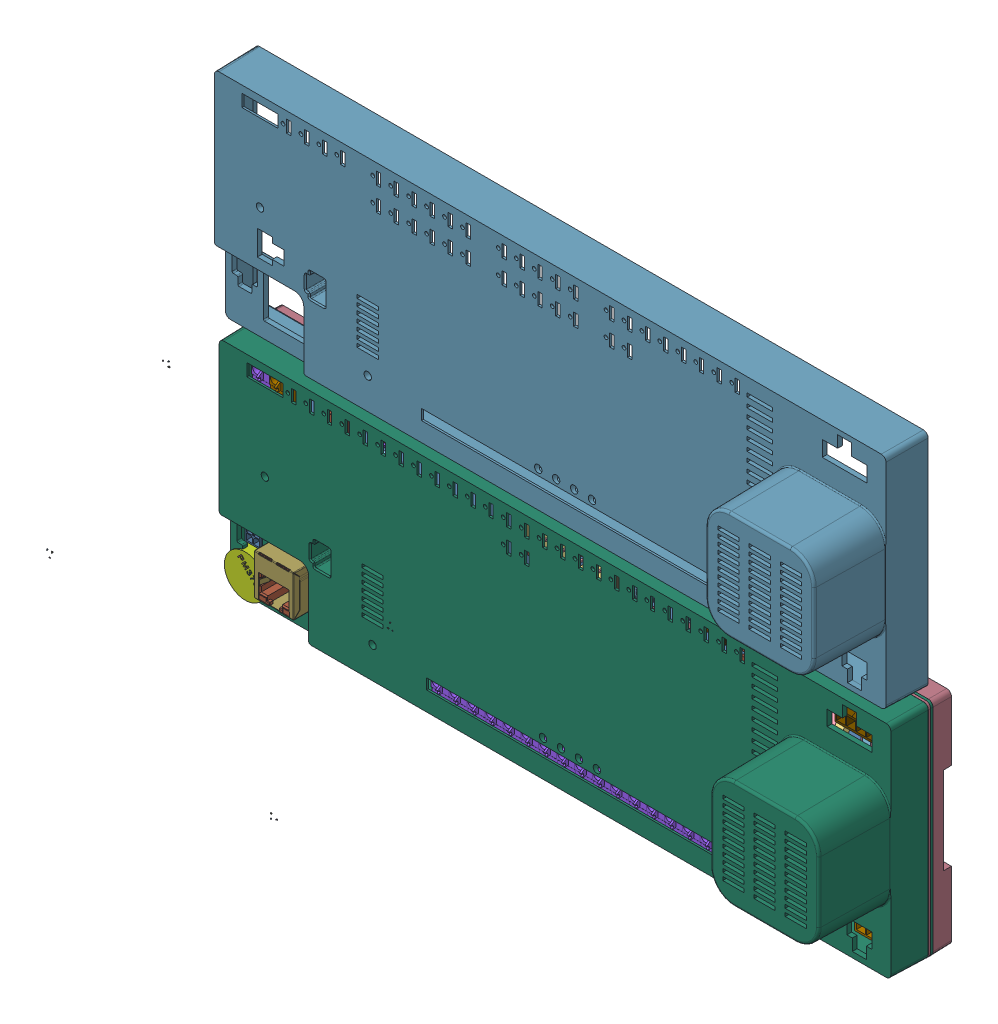
SolidWorks assembly _SC944D, configuration Default. Lengths in mm. (continued)
Components (placement in the parent): (continued)
- R2-1: R2 [Default] at origin size (0.8 1.6 0.55)
  - RESC1608X84N-1: RESC1608X84N [Default] at (41.4337 68.2626 0) x (0 1 0) z (1 0 0) size (1.6 0.55 0.8)
- R3-1: R3 [Default] at origin size (1.6 0.8 0.55)
  - RESC1608X84N-1: RESC1608X84N [Default] at (55.5308 79.4703 0) x (1 0 0) z (0 -1 0) size (1.6 0.55 0.8)
- R4-1: R4 [Default] at origin size (1.6 0.8 0.55)
  - RESC1608X84N-1: RESC1608X84N [Default] at (43.8151 70.9613 0) x (1 0 0) z (0 -1 0) size (1.6 0.55 0.8)
- R5-1: R5 [Default] at origin size (1.6 0.8 0.55)
  - RESC1608X84N-1: RESC1608X84N [Default] at (83.0262 24.4474 0) x (-1 0 0) z (0 1 0) size (1.6 0.55 0.8)
- R6-1: R6 [Default] at origin size (1.6 0.8 0.55)
  - RESC1608X84N-1: RESC1608X84N [Default] at (39.6876 53.8163 0) x (1 0 0) z (0 -1 0) size (1.6 0.55 0.8)
- R7-1: R7 [Default] at origin size (1.6 0.8 0.55)
  - RESC1608X84N-1: RESC1608X84N [Default] at (97.4091 78.7401 0) x (1 0 0) z (0 -1 0) size (1.6 0.55 0.8)
- R8-1: R8 [Default] at origin size (1.6 0.8 0.55)
  - RESC1608X84N-1: RESC1608X84N [Default] at (97.4089 76.9619 0) x (-1 0 0) z (0 1 0) size (1.6 0.55 0.8)
- R9-1: R9 [Default] at origin size (3.2 1.6 0.84)
  - RESC3216X84N-1: RESC3216X84N [Default] at (57.7849 61.1187 0) x (-1 0 0) z (0 1 0) size (3.2 0.84 1.6)
- R10-1: R10 [Default] at origin size (1.6 0.8 0.55)
  - RESC1608X84N-1: RESC1608X84N [Default] at (29.2099 4.2862 0) x (-1 0 0) z (0 1 0) size (1.6 0.55 0.8)
- R11-1: R11 [Default] at origin size (1.6 0.8 0.55)
  - RESC1608X84N-1: RESC1608X84N [Default] at (146.0499 57.5309 0) x (-1 0 0) z (0 1 0) size (1.6 0.55 0.8)
- R12-1: R12 [Default] at origin size (1.6 0.8 0.55)
  - RESC1608X84N-1: RESC1608X84N [Default] at (115.0619 55.7529 0) x (-1 0 0) z (0 1 0) size (1.6 0.55 0.8)
- R14-1: R14 [Default] at origin size (1.6 0.8 0.55)
  - RESC1608X84N-1: RESC1608X84N [Default] at (120.7769 63.2459 0) x (-1 0 0) z (0 1 0) size (1.6 0.55 0.8)
- R15-1: R15 [Default] at origin size (0.8 1.6 0.55)
  - RESC1608X84N-1: RESC1608X84N [Default] at (118.3641 63.8809 0) x (0 -1 0) z (-1 0 0) size (1.6 0.55 0.8)
- R16-1: R16 [Default] at origin size (1.6 0.8 0.55)
  - RESC1608X84N-1: RESC1608X84N [Default] at (29.2099 2.5399 0) x (-1 0 0) z (0 1 0) size (1.6 0.55 0.8)
- R17-1: R17 [Default] at origin size (1.6 0.8 0.55)
  - RESC1608X84N-1: RESC1608X84N [Default] at (143.3831 50.6731 0) x (1 0 0) z (0 -1 0) size (1.6 0.55 0.8)
- R18-1: R18 [Default] at origin size (0.8 1.6 0.55)
  - RESC1608X84N-1: RESC1608X84N [Default] at (121.6661 53.7209 0) x (0 -1 0) z (-1 0 0) size (1.6 0.55 0.8)
- R19-1: R19 [Default] at origin size (3.2 1.6 0.84)
  - RESC3216X84N-1: RESC3216X84N [Default] at (110.1724 8.8899 0) x (-1 0 0) z (0 1 0) size (3.2 0.84 1.6)
- R20-1: R20 [Default] at origin size (3.2 1.6 0.84)
  - RESC3216X84N-1: RESC3216X84N [Default] at (110.2359 24.7649 0) x (-1 0 0) z (0 1 0) size (3.2 0.84 1.6)
- R21-1: R21 [Default] at origin size (1.6 0.8 0.55)
  - RESC1608X84N-1: RESC1608X84N [Default] at (119.1261 50.4191 0) x (1 0 0) z (0 -1 0) size (1.6 0.55 0.8)
- R22-1: R22 [Default] at origin size (1.6 0.8 0.55)
  - RESC1608X84N-1: RESC1608X84N [Default] at (39.6874 61.2775 0) x (-1 0 0) z (0 1 0) size (1.6 0.55 0.8)
- R23-1: R23 [Default] at origin size (1.6 0.8 0.55)
  - RESC1608X84N-1: RESC1608X84N [Default] at (200.5649 35.4012 0) x (-1 0 0) z (0 1 0) size (1.6 0.55 0.8)
- R24-1: R24 [Default] at origin size (6.4 3.2 0.7)
  - RESC6432X76N-1: RESC6432X76N [Default] at (160.782 62.4839 0) x (-1 0 0) z (0 1 0) size (6.4 0.7 3.2)
- R25-1: R25 [Default] at origin size (0.8 1.6 0.55)
  - RESC1608X84N-1: RESC1608X84N [Default] at (162.0521 66.6749 0) x (0 -1 0) z (-1 0 0) size (1.6 0.55 0.8)
- R26-1: R26 [Default] at origin size (1.6 0.8 0.55)
  - RESC1608X84N-1: RESC1608X84N [Default] at (162.6869 73.5329 0) x (-1 0 0) z (0 1 0) size (1.6 0.55 0.8)
- R27-1: R27 [Default] at origin size (0.8 1.6 0.55)
  - RESC1608X84N-1: RESC1608X84N [Default] at (80.3276 25.0824 0) x (0 -1 0) z (-1 0 0) size (1.6 0.55 0.8)
- R28-1: R28 [Default] at origin size (6.4 3.2 0.7)
  - RESC6432X76N-1: RESC6432X76N [Default] at (180.0861 65.9131 0) x (1 0 0) z (0 -1 0) size (6.4 0.7 3.2)
- R29-1: R29 [Default] at origin size (1.6 0.8 0.55)
  - RESC1608X84N-1: RESC1608X84N [Default] at (186.0549 70.866 0) x (-1 0 0) z (0 1 0) size (1.6 0.55 0.8)
- R30-1: R30 [Default] at origin size (1.6 0.8 0.55)
  - RESC1608X84N-1: RESC1608X84N [Default] at (189.1029 70.866 0) x (-1 0 0) z (0 1 0) size (1.6 0.55 0.8)
- R31-1: R31 [Default] at origin size (0.8 1.6 0.55)
  - RESC1608X84N-1: RESC1608X84N [Default] at (35.0838 21.4312 0) x (0 -1 0) z (-1 0 0) size (1.6 0.55 0.8)
- R32-1: R32 [Default] at origin size (1.6 0.8 0.55)
  - RESC1608X84N-1: RESC1608X84N [Default] at (82.8676 30.1626 0) x (1 0 0) z (0 -1 0) size (1.6 0.55 0.8)
- R33-1: R33 [Default] at origin size (0.8 1.6 0.55)
  - RESC1608X84N-1: RESC1608X84N [Default] at (57.9437 58.2613 0) x (0 1 0) z (1 0 0) size (1.6 0.55 0.8)
- R34-1: R34 [Default] at origin size (1.6 0.8 0.55)
  - RESC1608X84N-1: RESC1608X84N [Default] at (139.0649 50.7288 0) x (-1 0 0) z (0 1 0) size (1.6 0.55 0.8)
- R37-1: R37 [Default] at origin size (3.2 1.6 0.84)
  - RESC3216X84N-1: RESC3216X84N [Default] at (136.9059 57.9678 0) x (-1 0 0) z (0 1 0) size (3.2 0.84 1.6)
- R39-1: R39 [Default] at origin size (1.6 0.8 0.55)
  - RESC1608X84N-1: RESC1608X84N [Default] at (78.7401 11.7475 0) x (1 0 0) z (0 -1 0) size (1.6 0.55 0.8)
- R41-1: R41 [Default] at origin size (1.6 0.8 0.55)
  - RESC1608X84N-1: RESC1608X84N [Default] at (107.0609 27.8129 0) x (-1 0 0) z (0 1 0) size (1.6 0.55 0.8)
- R42-1: R42 [Default] at origin size (1.6 0.8 0.55)
  - RESC1608X84N-1: RESC1608X84N [Default] at (24.7649 33.9724 0) x (-1 0 0) z (0 1 0) size (1.6 0.55 0.8)
- R43-1: R43 [Default] at origin size (1.6 0.8 0.55)
  - RESC1608X84N-1: RESC1608X84N [Default] at (27.1462 51.435 0) x (-1 0 0) z (0 1 0) size (1.6 0.55 0.8)
- R44-1: R44 [Default] at origin size (0.8 1.6 0.55)
  - RESC1608X84N-1: RESC1608X84N [Default] at (28.5749 44.6088 0) x (0 1 0) z (1 0 0) size (1.6 0.55 0.8)
- R45-1: R45 [Default] at origin size (1.6 0.8 0.55)
  - RESC1608X84N-1: RESC1608X84N [Default] at (36.6712 53.8162 0) x (-1 0 0) z (0 1 0) size (1.6 0.55 0.8)
- R46-1: R46 [Default] at origin size (1.6 0.8 0.55)
  - RESC1608X84N-1: RESC1608X84N [Default] at (31.5912 47.625 0) x (-1 0 0) z (0 1 0) size (1.6 0.55 0.8)
- R47-1: R47 [Default] at origin size (1.6 0.8 0.55)
  - RESC1608X84N-1: RESC1608X84N [Default] at (73.8188 20.955 0) x (1 0 0) z (0 -1 0) size (1.6 0.55 0.8)
- R48-1: R48 [Default] at origin size (1.6 0.8 0.55)
  - RESC1608X84N-1: RESC1608X84N [Default] at (67.1513 9.6838 0) x (1 0 0) z (0 -1 0) size (1.6 0.55 0.8)
- R49-1: R49 [Default] at origin size (1.6 0.8 0.55)
  - RESC1608X84N-1: RESC1608X84N [Default] at (9.0488 62.5475 0) x (1 0 0) z (0 -1 0) size (1.6 0.55 0.8)
- R50-1: R50 [Default] at origin size (0.8 1.6 0.55)
  - RESC1608X84N-1: RESC1608X84N [Default] at (33.3376 52.2287 0) x (0 -1 0) z (-1 0 0) size (1.6 0.55 0.8)
- R51-1: R51 [Default] at origin size (0.8 1.6 0.55)
  - RESC1608X84N-1: RESC1608X84N [Default] at (83.566 41.7831 0) x (0 1 0) z (1 0 0) size (1.6 0.55 0.8)
- R52-1: R52 [Default] at origin size (0.8 1.6 0.55)
  - RESC1608X84N-1: RESC1608X84N [Default] at (100.7109 38.9891 0) x (0 1 0) z (1 0 0) size (1.6 0.55 0.8)
- R53-1: R53 [Default] at origin size (1.6 0.8 0.55)
  - RESC1608X84N-1: RESC1608X84N [Default] at (21.9076 37.9413 0) x (1 0 0) z (0 -1 0) size (1.6 0.55 0.8)
- R54-1: R54 [Default] at origin size (1.6 0.8 0.55)
  - RESC1608X84N-1: RESC1608X84N [Default] at (170.5611 79.248 0) x (1 0 0) z (0 -1 0) size (1.6 0.55 0.8)
- R55-1: R55 [Default] at origin size (1.6 0.8 0.55)
  - RESC1608X84N-1: RESC1608X84N [Default] at (173.7361 77.47 0) x (1 0 0) z (0 -1 0) size (1.6 0.55 0.8)
- R56-1: R56 [Default] at origin size (1.6 0.8 0.55)
  - RESC1608X84N-1: RESC1608X84N [Default] at (233.3626 27.4638 0) x (1 0 0) z (0 -1 0) size (1.6 0.55 0.8)
- R57-1: R57 [Default] at origin size (0.8 1.6 0.55)
  - RESC1608X84N-1: RESC1608X84N [Default] at (83.566 48.5496 0) x (0 1 0) z (1 0 0) size (1.6 0.55 0.8)
- R58-1: R58 [Default] at origin size (1.6 0.8 0.55)
  - RESC1608X84N-1: RESC1608X84N [Default] at (103.5049 34.1629 0) x (-1 0 0) z (0 1 0) size (1.6 0.55 0.8)
- R59-1: R59 [Default] at origin size (0.8 1.6 0.55)
  - RESC1608X84N-1: RESC1608X84N [Default] at (189.8488 36.2305 0) x (0 -1 0) z (-1 0 0) size (1.6 0.55 0.8)
- R60-1: R60 [Default] at origin size (1.6 0.8 0.55)
  - RESC1608X84N-1: RESC1608X84N [Default] at (107.0609 34.1629 0) x (-1 0 0) z (0 1 0) size (1.6 0.55 0.8)
- R61-1: R61 [Default] at origin size (0.8 1.6 0.55)
  - RESC1608X84N-1: RESC1608X84N [Default] at (240.5062 77.3113 0) x (0 1 0) z (1 0 0) size (1.6 0.55 0.8)
- R62-1: R62 [Default] at origin size (0.8 1.6 0.55)
  - RESC1608X84N-1: RESC1608X84N [Default] at (11.4301 62.8649 0) x (0 -1 0) z (-1 0 0) size (1.6 0.55 0.8)
- R63-1: R63 [Default] at origin size (0.8 1.6 0.55)
  - RESC1608X84N-1: RESC1608X84N [Default] at (230.775 77.9781 0) x (0 1 0) z (1 0 0) size (1.6 0.55 0.8)
- R65-1: R65 [Default] at origin size (1.6 0.8 0.55)
  - RESC1608X84N-1: RESC1608X84N [Default] at (233.3624 25.8762 0) x (-1 0 0) z (0 1 0) size (1.6 0.55 0.8)
- R66-1: R66 [Default] at origin size (0.8 1.6 0.55)
  - RESC1608X84N-1: RESC1608X84N [Default] at (193.8337 52.7051 0) x (0 1 0) z (1 0 0) size (1.6 0.55 0.8)
- R67-1: R67 [Default] at origin size (1.6 0.8 0.55)
  - RESC1608X84N-1: RESC1608X84N [Default] at (243.0462 76.6762 0) x (-1 0 0) z (0 1 0) size (1.6 0.55 0.8)
- R68-1: R68 [Default] at origin size (1.6 0.8 0.55)
  - RESC1608X84N-1: RESC1608X84N [Default] at (244.4749 74.144 0) x (-1 0 0) z (0 1 0) size (1.6 0.55 0.8)
- R69-1: R69 [Default] at origin size (0.8 1.6 0.55)
  - RESC1608X84N-1: RESC1608X84N [Default] at (234.4738 72.0724 0) x (0 -1 0) z (-1 0 0) size (1.6 0.55 0.8)
- R70-1: R70 [Default] at origin size (1.6 0.8 0.55)
  - RESC1608X84N-1: RESC1608X84N [Default] at (230.8224 67.7862 0) x (-1 0 0) z (0 1 0) size (1.6 0.55 0.8)
- R71-1: R71 [Default] at origin size (0.8 1.6 0.55)
  - RESC1608X84N-1: RESC1608X84N [Default] at (36.8299 21.4313 0) x (0 1 0) z (1 0 0) size (1.6 0.55 0.8)
- R72-1: R72 [Default] at origin size (1.6 0.8 0.55)
  - RESC1608X84N-1: RESC1608X84N [Default] at (29.7179 18.161 0) x (-1 0 0) z (0 1 0) size (1.6 0.55 0.8)
- R73-1: R73 [Default] at origin size (1.6 0.8 0.55)
  - RESC1608X84N-1: RESC1608X84N [Default] at (37.0244 6.8263 0) x (1 0 0) z (0 -1 0) size (1.6 0.55 0.8)
- R74-1: R74 [Default] at origin size (0.8 1.6 0.55)
  - RESC1608X84N-1: RESC1608X84N [Default] at (202.7238 61.1187 0) x (0 -1 0) z (-1 0 0) size (1.6 0.55 0.8)
- R75-1: R75 [Default] at origin size (0.8 1.6 0.55)
  - RESC1608X84N-1: RESC1608X84N [Default] at (41.783 20.9549 0) x (0 -1 0) z (-1 0 0) size (1.6 0.55 0.8)
- R76-1: R76 [Default] at origin size (0.8 1.6 0.55)
  - RESC1608X84N-1: RESC1608X84N [Default] at (34.1313 44.1324 0) x (0 -1 0) z (-1 0 0) size (1.6 0.55 0.8)
- R77-1: R77 [Default] at origin size (1.6 0.8 0.55)
  - RESC1608X84N-1: RESC1608X84N [Default] at (29.7179 16.6369 0) x (-1 0 0) z (0 1 0) size (1.6 0.55 0.8)
- R78-1: R78 [Default] at origin size (1.6 0.8 0.55)
  - RESC1608X84N-1: RESC1608X84N [Default] at (29.7179 15.1129 0) x (-1 0 0) z (0 1 0) size (1.6 0.55 0.8)
- R79-1: R79 [Default] at origin size (1.6 0.8 0.55)
  - RESC1608X84N-1: RESC1608X84N [Default] at (29.7179 13.5889 0) x (-1 0 0) z (0 1 0) size (1.6 0.55 0.8)
- R80-1: R80 [Default] at origin size (1.6 0.8 0.55)
  - RESC1608X84N-1: RESC1608X84N [Default] at (27.1463 42.2276 0) x (1 0 0) z (0 -1 0) size (1.6 0.55 0.8)
- R81-1: R81 [Default] at origin size (1.6 0.8 0.55)
  - RESC1608X84N-1: RESC1608X84N [Default] at (27.1463 53.3401 0) x (1 0 0) z (0 -1 0) size (1.6 0.55 0.8)
- R82-1: R82 [Default] at origin size (1.6 0.8 0.55)
  - RESC1608X84N-1: RESC1608X84N [Default] at (73.6601 33.528 0) x (1 0 0) z (0 -1 0) size (1.6 0.55 0.8)
- R83-1: R83 [Default] at origin size (1.6 0.8 0.55)
  - RESC1608X84N-1: RESC1608X84N [Default] at (73.6601 32.004 0) x (1 0 0) z (0 -1 0) size (1.6 0.55 0.8)
- R84-1: R84 [Default] at origin size (1.6 0.8 0.55)
  - RESC1608X84N-1: RESC1608X84N [Default] at (40.2715 6.8419 0) x (1 0 0) z (0 -1 0) size (1.6 0.55 0.8)
- R85-1: R85 [Default] at origin size (1.6 0.8 0.55)
  - RESC1608X84N-1: RESC1608X84N [Default] at (29.7181 10.541 0) x (1 0 0) z (0 -1 0) size (1.6 0.55 0.8)
- R35-1: R35 [Default] at origin size (0.8 1.6 0.55)
  - RESC1608X84N-1: RESC1608X84N [Default] at (100.7109 32.6391 0) x (0 1 0) z (1 0 0) size (1.6 0.55 0.8)
- R87-1: R87 [Default] at origin size (1.6 0.8 0.55)
  - RESC1608X84N-1: RESC1608X84N [Default] at (86.2331 34.4171 0) x (1 0 0) z (0 -1 0) size (1.6 0.55 0.8)
- R88-1: R88 [Default] at origin size (1.6 0.8 0.55)
  - RESC1608X84N-1: RESC1608X84N [Default] at (192.2139 49.3712 0) x (-1 0 0) z (0 1 0) size (1.6 0.55 0.8)
- R90-1: R90 [Default] at origin size (1.6 0.8 0.55)
  - RESC1608X84N-1: RESC1608X84N [Default] at (107.0609 40.64 0) x (-1 0 0) z (0 1 0) size (1.6 0.55 0.8)
- R91-1: R91 [Default] at origin size (1.6 0.8 0.55)
  - RESC1608X84N-1: RESC1608X84N [Default] at (226.6594 70.993 0) x (-1 0 0) z (0 1 0) size (1.6 0.55 0.8)
- R92-1: R92 [Default] at origin size (0.8 1.6 0.55)
  - RESC1608X84N-1: RESC1608X84N [Default] at (100.7109 51.6891 0) x (0 1 0) z (1 0 0) size (1.6 0.55 0.8)
- R93-1: R93 [Default] at origin size (1.6 0.8 0.55)
  - RESC1608X84N-1: RESC1608X84N [Default] at (103.5049 46.9899 0) x (-1 0 0) z (0 1 0) size (1.6 0.55 0.8)
- R95-1: R95 [Default] at origin size (0.8 1.6 0.55)
  - RESC1608X84N-1: RESC1608X84N [Default] at (230.1875 70.0088 0) x (0 1 0) z (1 0 0) size (1.6 0.55 0.8)
- R97-1: R97 [Default] at origin size (0.8 1.6 0.55)
  - RESC1608X84N-1: RESC1608X84N [Default] at (81.407 38.7349 0) x (0 -1 0) z (-1 0 0) size (1.6 0.55 0.8)
- R100-1: R100 [Default] at origin size (0.8 1.6 0.55)
  - RESC1608X84N-1: RESC1608X84N [Default] at (81.407 42.2054 0) x (0 -1 0) z (-1 0 0) size (1.6 0.55 0.8)
- R103-1: R103 [Default] at origin size (1.6 0.8 0.55)
  - RESC1608X84N-1: RESC1608X84N [Default] at (51.5226 53.9749 0) x (-1 0 0) z (0 1 0) size (1.6 0.55 0.8)
- R104-1: R104 [Default] at origin size (0.8 1.6 0.55)
  - RESC1608X84N-1: RESC1608X84N [Default] at (54.7688 44.7674 0) x (0 -1 0) z (-1 0 0) size (1.6 0.55 0.8)
- R106-1: R106 [Default] at origin size (1.6 0.8 0.55)
  - RESC1608X84N-1: RESC1608X84N [Default] at (44.4499 40.4812 0) x (-1 0 0) z (0 1 0) size (1.6 0.55 0.8)
- R107-1: R107 [Default] at origin size (0.8 1.6 0.55)
  - RESC1608X84N-1: RESC1608X84N [Default] at (69.6912 41.7513 0) x (0 1 0) z (1 0 0) size (1.6 0.55 0.8)
- R108-1: R108 [Default] at origin size (0.8 1.6 0.55)
  - RESC1608X84N-1: RESC1608X84N [Default] at (57.1501 1.5874 0) x (0 -1 0) z (-1 0 0) size (1.6 0.55 0.8)
- R109-1: R109 [Default] at origin size (1.6 0.8 0.55)
  - RESC1608X84N-1: RESC1608X84N [Default] at (54.7687 0.9524 0) x (-1 0 0) z (0 1 0) size (1.6 0.55 0.8)
- R110-1: R110 [Default] at origin size (1.6 0.8 0.55)
  - RESC1608X84N-1: RESC1608X84N [Default] at (51.7524 0.9524 0) x (-1 0 0) z (0 1 0) size (1.6 0.55 0.8)
- R111-1: R111 [Default] at origin size (2 1.2 0.7)
  - RESC2012X70N-1: RESC2012X70N [Default] at (63.7541 37.3381 0) x (1 0 0) z (0 -1 0) size (2 0.7 1.2)
- R112-1: R112 [Default] at origin size (0.8 1.6 0.55)
  - RESC1608X84N-1: RESC1608X84N [Default] at (46.8986 35.3415 0) x (0 -1 0) z (-1 0 0) size (1.6 0.55 0.8)
- R113-1: R113 [Default] at origin size (1.6 0.8 0.55)
  - RESC1608X84N-1: RESC1608X84N [Default] at (43.0212 31.1149 0) x (-1 0 0) z (0 1 0) size (1.6 0.55 0.8)
- R115-1: R115 [Default] at origin size (1.6 0.8 0.55)
  - RESC1608X84N-1: RESC1608X84N [Default] at (215.9356 38.989 0) x (1 0 0) z (0 -1 0) size (1.6 0.55 0.8)
- R116-1: R116 [Default] at origin size (0.8 1.6 0.55)
  - RESC1608X84N-1: RESC1608X84N [Default] at (200.1837 61.1188 0) x (0 1 0) z (1 0 0) size (1.6 0.55 0.8)
- R121-1: R121 [Default] at origin size (1.6 0.8 0.55)
  - RESC1608X84N-1: RESC1608X84N [Default] at (86.2331 40.767 0) x (1 0 0) z (0 -1 0) size (1.6 0.55 0.8)
- R125-1: R125 [Default] at origin size (0.8 1.6 0.55)
  - RESC1608X84N-1: RESC1608X84N [Default] at (203.9937 42.3863 0) x (0 1 0) z (1 0 0) size (1.6 0.55 0.8)
- R129-1: R129 [Default] at origin size (0.8 1.6 0.55)
  - RESC1608X84N-1: RESC1608X84N [Default] at (70.1751 53.9749 0) x (0 -1 0) z (-1 0 0) size (1.6 0.55 0.8)
- R137-1: R137 [Default] at origin size (1.6 0.8 0.55)
  - RESC1608X84N-1: RESC1608X84N [Default] at (86.2331 47.1171 0) x (1 0 0) z (0 -1 0) size (1.6 0.55 0.8)
- R141-1: R141 [Default] at origin size (1.6 0.8 0.55)
  - RESC1608X84N-1: RESC1608X84N [Default] at (49.3116 4.6991 0) x (1 0 0) z (0 -1 0) size (1.6 0.55 0.8)
- R145-1: R145 [Default] at origin size (1.6 0.8 0.55)
  - RESC1608X84N-1: RESC1608X84N [Default] at (76.4541 54.483 0) x (1 0 0) z (0 -1 0) size (1.6 0.55 0.8)
- R153-1: R153 [Default] at origin size (1.6 0.8 0.55)
  - RESC1608X84N-1: RESC1608X84N [Default] at (86.3601 53.4671 0) x (1 0 0) z (0 -1 0) size (1.6 0.55 0.8)
- R154-1: R154 [Default] at origin size (0.8 1.6 0.55)
  - RESC1608X84N-1: RESC1608X84N [Default] at (1.5241 22.3519 0) x (0 -1 0) z (-1 0 0) size (1.6 0.55 0.8)
- R155-1: R155 [Default] at origin size (1.6 0.8 0.55)
  - RESC1608X84N-1: RESC1608X84N [Default] at (4.0639 20.955 0) x (-1 0 0) z (0 1 0) size (1.6 0.55 0.8)
- R156-1: R156 [Default] at origin size (1.6 0.8 0.55)
  - RESC1608X84N-1: RESC1608X84N [Default] at (6.9851 20.955 0) x (1 0 0) z (0 -1 0) size (1.6 0.55 0.8)
- R157-1: R157 [Default] at origin size (1.6 0.8 0.55)
  - RESC1608X84N-1: RESC1608X84N [Default] at (10.3785 23.4951 0) x (1 0 0) z (0 -1 0) size (1.6 0.55 0.8)
- R158-1: R158 [Default] at origin size (1.6 0.8 0.55)
  - RESC1608X84N-1: RESC1608X84N [Default] at (10.3785 25.1461 0) x (1 0 0) z (0 -1 0) size (1.6 0.55 0.8)
- R168-1: R168 [Default] at origin size (1.6 0.8 0.55)
  - RESC1608X84N-1: RESC1608X84N [Default] at (76.4539 56.642 0) x (-1 0 0) z (0 1 0) size (1.6 0.55 0.8)
- R176-1: R176 [Default] at origin size (1.6 0.8 0.55)
  - RESC1608X84N-1: RESC1608X84N [Default] at (214.1537 35.4012 0) x (-1 0 0) z (0 1 0) size (1.6 0.55 0.8)
- R177-1: R177 [Default] at origin size (0.8 1.6 0.55)
  - RESC1608X84N-1: RESC1608X84N [Default] at (205.4224 68.2626 0) x (0 1 0) z (1 0 0) size (1.6 0.55 0.8)
- R179-1: R179 [Default] at origin size (1.6 0.8 0.55)
  - RESC1608X84N-1: RESC1608X84N [Default] at (148.3361 50.6731 0) x (1 0 0) z (0 -1 0) size (1.6 0.55 0.8)
- R184-1: R184 [Default] at origin size (0.8 1.6 0.55)
  - RESC1608X84N-1: RESC1608X84N [Default] at (197.4849 57.4041 0) x (0 1 0) z (1 0 0) size (1.6 0.55 0.8)
- R185-1: R185 [Default] at origin size (0.8 1.6 0.55)
  - RESC1608X84N-1: RESC1608X84N [Default] at (202.6919 57.2771 0) x (0 1 0) z (1 0 0) size (1.6 0.55 0.8)
- R186-1: R186 [Default] at origin size (1.6 3.2 0.84)
  - RESC3216X84N-1: RESC3216X84N [Default] at (208.4071 54.9909 0) x (0 -1 0) z (-1 0 0) size (3.2 0.84 1.6)
- R189-1: R189 [Default] at origin size (0.8 1.6 0.55)
  - RESC1608X84N-1: RESC1608X84N [Default] at (205.2637 61.1188 0) x (0 1 0) z (1 0 0) size (1.6 0.55 0.8)
- R190-1: R190 [Default] at origin size (0.8 1.6 0.55)
  - RESC1608X84N-1: RESC1608X84N [Default] at (212.7249 54.2926 0) x (0 1 0) z (1 0 0) size (1.6 0.55 0.8)
- R191-1: R191 [Default] at origin size (1.6 0.8 0.55)
  - RESC1608X84N-1: RESC1608X84N [Default] at (12.0651 65.0876 0) x (1 0 0) z (0 -1 0) size (1.6 0.55 0.8)
- R193-1: R193 [Default] at origin size (1.6 0.8 0.55)
  - RESC1608X84N-1: RESC1608X84N [Default] at (14.4463 70.485 0) x (1 0 0) z (0 -1 0) size (1.6 0.55 0.8)
- R194-1: R194 [Default] at origin size (0.8 1.6 0.55)
  - RESC1608X84N-1: RESC1608X84N [Default] at (14.6049 57.7851 0) x (0 1 0) z (1 0 0) size (1.6 0.55 0.8)
- R195-1: R195 [Default] at origin size (6.5 23.66 10.15)
  - User_Library-RES-3W-1: User_Library-RES-3W [Default] at (0.0002 75.1651 0) x (0 -1 0) z (0 0 1) size (23.66 6.5 10.15)
    - User_Library-RES-3W_RES_3W002-1: User_Library-RES-3W_RES_3W002 [Default] at origin size (17.5 6.5 7.8)
    - User_Library-RES-3W_RES_3W005-1: User_Library-RES-3W_RES_3W005 [Default] at origin size (1 6.24 6.24)
    - User_Library-RES-3W_RES_3W003-1: User_Library-RES-3W_RES_3W003 [Default] at origin size (1 6.24 6.24)
    - User_Library-RES-3W_RES_3W004-1: User_Library-RES-3W_RES_3W004 [Default] at origin size (1 6.24 6.24)
    - User_Library-RES-3W_Fusion-1: User_Library-RES-3W_Fusion [Default] at origin size (3.18 0.8 6.65)
    - User_Library-RES-3W_Fusion_1-1: User_Library-RES-3W_Fusion_1 [Default] at origin size (3.18 0.8 6.65)
    - User_Library-RES-3W_RES_3W006-1: User_Library-RES-3W_RES_3W006 [Default] at origin size (1 6.24 6.24)
- R196-1: R196 [Default] at origin size (0.8 1.6 0.55)
  - RESC1608X84N-1: RESC1608X84N [Default] at (12.6999 54.1338 0) x (0 1 0) z (1 0 0) size (1.6 0.55 0.8)
- R197-1: R197 [Default] at origin size (1.6 0.8 0.55)
  - RESC1608X84N-1: RESC1608X84N [Default] at (8.0963 57.1501 0) x (1 0 0) z (0 -1 0) size (1.6 0.55 0.8)
- R198-1: R198 [Default] at origin size (1.6 0.8 0.55)
  - RESC1608X84N-1: RESC1608X84N [Default] at (9.8424 67.31 0) x (-1 0 0) z (0 1 0) size (1.6 0.55 0.8)
- R199-1: R199 [Default] at origin size (1.6 0.8 0.55)
  - RESC1608X84N-1: RESC1608X84N [Default] at (6.1912 64.1349 0) x (-1 0 0) z (0 1 0) size (1.6 0.55 0.8)
- R201-1: R201 [Default] at origin size (0.8 1.6 0.55)
  - RESC1608X84N-1: RESC1608X84N [Default] at (5.5562 61.7538 0) x (0 1 0) z (1 0 0) size (1.6 0.55 0.8)
- R202-1: R202 [Default] at origin size (0.8 1.6 0.55)
  - RESC1608X84N-1: RESC1608X84N [Default] at (210.8199 54.2926 0) x (0 1 0) z (1 0 0) size (1.6 0.55 0.8)
- R204-1: R204 [Default] at origin size (1.6 0.8 0.55)
  - RESC1608X84N-1: RESC1608X84N [Default] at (197.8024 49.2124 0) x (-1 0 0) z (0 1 0) size (1.6 0.55 0.8)
- R205-1: R205 [Default] at origin size (1.6 0.8 0.55)
  - RESC1608X84N-1: RESC1608X84N [Default] at (204.8511 49.657 0) x (1 0 0) z (0 -1 0) size (1.6 0.55 0.8)
- R207-1: R207 [Default] at origin size (1.6 0.8 0.55)
  - RESC1608X84N-1: RESC1608X84N [Default] at (204.8509 51.435 0) x (-1 0 0) z (0 1 0) size (1.6 0.55 0.8)
- R208-1: R208 [Default] at origin size (1.6 0.8 0.55)
  - RESC1608X84N-1: RESC1608X84N [Default] at (197.8026 51.435 0) x (1 0 0) z (0 -1 0) size (1.6 0.55 0.8)
- RR1-1: RR1 [Default] at origin size (3.2 1.6 0.58)
  - User_Library-R1206-4R-1: User_Library-R1206-4R [Default] at (73.88 3.4552 -3.35) x (0 -1 0) z (-1 0 0) size (1.6 0.58 3.2)
- RR2-1: RR2 [Default] at origin size (1.6 3.2 0.58)
  - User_Library-R1206-4R-1: User_Library-R1206-4R [Default] at (56.4508 13.866 -3.35) x (1 0 0) z (0 -1 0) size (1.6 0.58 3.2)
- RR3-1: RR3 [Default] at origin size (1.6 3.2 0.58)
  - User_Library-R1206-4R-1: User_Library-R1206-4R [Default] at (56.4379 9.7958 -3.35) x (1 0 0) z (0 -1 0) size (1.6 0.58 3.2)
- T1-1: T1 [Default] at origin size (9.94 6.54 2.42)
  - SW3dPS-DPAK-1-1: SW3dPS-DPAK-1 [Default] at (50.3209 61.1662 1.2) x (0 1 0) z (1 0 0) size (6.54 2.42 9.94)
- T2-1: T2 [Default] at origin size (173.64 21.68 23.48)
  - SW3dPS-transistor_SOT233-1: SW3dPS-transistor_SOT233 [Default] at (170.7698 -18.1992 -21.9) x (0 -1 0) z (-1 0 0) size (2.9 1.1 1.6)
  - SW3dPS-transistor_SOT233_1-1: SW3dPS-transistor_SOT233_1 [Default] at (0.1708 -0.0182 -0.0219) x (0 -1 0) z (-1 0 0) size (2.18 2.18 2.18)
  - SW3dPS-transistor_SOT233_2-1: SW3dPS-transistor_SOT233_2 [Default] at (0.0002 0 0) x (0 -1 0) z (-1 0 0) size (2.18 2.18 2.18)
  - SW3dPS-transistor_SOT233_3-1: SW3dPS-transistor_SOT233_3 [Default] x (0 -1 0) z (-1 0 0) size (2.18 2.18 2.18)
- T3-1: T3 [Default] at origin size (83.82 106.77 23.48)
  - SW3dPS-transistor_SOT233-1: SW3dPS-transistor_SOT233 [Default] at (80.9442 103.2892 -21.9) x (0 1 0) z (1 0 0) size (2.9 1.1 1.6)
  - SW3dPS-transistor_SOT233_1-1: SW3dPS-transistor_SOT233_1 [Default] at (0.0809 0.1033 -0.0219) x (0 1 0) z (1 0 0) size (2.18 2.18 2.18)
  - SW3dPS-transistor_SOT233_2-1: SW3dPS-transistor_SOT233_2 [Default] at (0.0001 0.0001 0) x (0 1 0) z (1 0 0) size (2.18 2.18 2.18)
  - SW3dPS-transistor_SOT233_3-1: SW3dPS-transistor_SOT233_3 [Default] x (0 1 0) z (1 0 0) size (2.18 2.18 2.18)
- T4-1: T4 [Default] at origin size (9.94 6.54 2.42)
  - SW3dPS-DPAK-1-1: SW3dPS-DPAK-1 [Default] at (130.2283 52.9849 1.2) x (0 1 0) z (1 0 0) size (6.54 2.42 9.94)
- T5-1: T5 [Default] at origin size (169.58 21.68 23.48)
  - SW3dPS-transistor_SOT233-1: SW3dPS-transistor_SOT233 [Default] at (166.7058 -18.1992 -21.9) x (0 -1 0) z (-1 0 0) size (2.9 1.1 1.6)
  - SW3dPS-transistor_SOT233_1-1: SW3dPS-transistor_SOT233_1 [Default] at (0.1667 -0.0182 -0.0219) x (0 -1 0) z (-1 0 0) size (2.18 2.18 2.18)
  - SW3dPS-transistor_SOT233_2-1: SW3dPS-transistor_SOT233_2 [Default] at (0.0002 0 0) x (0 -1 0) z (-1 0 0) size (2.18 2.18 2.18)
  - SW3dPS-transistor_SOT233_3-1: SW3dPS-transistor_SOT233_3 [Default] x (0 -1 0) z (-1 0 0) size (2.18 2.18 2.18)
- T6-1: T6 [Default] at origin size (98.64 132.45 23.48)
  - SW3dPS-transistor_SOT233-1: SW3dPS-transistor_SOT233 [Default] at (95.7714 128.9749 -21.9) x (0 1 0) z (1 0 0) size (2.9 1.1 1.6)
  - SW3dPS-transistor_SOT233_1-1: SW3dPS-transistor_SOT233_1 [Default] at (0.0958 0.129 -0.0219) x (0 1 0) z (1 0 0) size (2.18 2.18 2.18)
  - SW3dPS-transistor_SOT233_2-1: SW3dPS-transistor_SOT233_2 [Default] at (0.0001 0.0001 0) x (0 1 0) z (1 0 0) size (2.18 2.18 2.18)
  - SW3dPS-transistor_SOT233_3-1: SW3dPS-transistor_SOT233_3 [Default] x (0 1 0) z (1 0 0) size (2.18 2.18 2.18)
- T7-1: T7 [Default] at origin size (83.82 113.12 23.48)
  - SW3dPS-transistor_SOT233-1: SW3dPS-transistor_SOT233 [Default] at (80.9442 109.6392 -21.9) x (0 1 0) z (1 0 0) size (2.9 1.1 1.6)
  - SW3dPS-transistor_SOT233_1-1: SW3dPS-transistor_SOT233_1 [Default] at (0.0809 0.1096 -0.0219) x (0 1 0) z (1 0 0) size (2.18 2.18 2.18)
  - SW3dPS-transistor_SOT233_2-1: SW3dPS-transistor_SOT233_2 [Default] at (0.0001 0.0001 0) x (0 1 0) z (1 0 0) size (2.18 2.18 2.18)
  - SW3dPS-transistor_SOT233_3-1: SW3dPS-transistor_SOT233_3 [Default] x (0 1 0) z (1 0 0) size (2.18 2.18 2.18)
- T8-1: T8 [Default] at origin size (83.82 119.47 23.48)
  - SW3dPS-transistor_SOT233-1: SW3dPS-transistor_SOT233 [Default] at (80.9442 115.9892 -21.9) x (0 1 0) z (1 0 0) size (2.9 1.1 1.6)
  - SW3dPS-transistor_SOT233_1-1: SW3dPS-transistor_SOT233_1 [Default] at (0.0809 0.116 -0.0219) x (0 1 0) z (1 0 0) size (2.18 2.18 2.18)
  - SW3dPS-transistor_SOT233_2-1: SW3dPS-transistor_SOT233_2 [Default] at (0.0001 0.0001 0) x (0 1 0) z (1 0 0) size (2.18 2.18 2.18)
  - SW3dPS-transistor_SOT233_3-1: SW3dPS-transistor_SOT233_3 [Default] x (0 1 0) z (1 0 0) size (2.18 2.18 2.18)
- T9-1: T9 [Default] at origin size (83.82 125.82 23.48)
  - SW3dPS-transistor_SOT233-1: SW3dPS-transistor_SOT233 [Default] at (80.9442 122.3392 -21.9) x (0 1 0) z (1 0 0) size (2.9 1.1 1.6)
  - SW3dPS-transistor_SOT233_1-1: SW3dPS-transistor_SOT233_1 [Default] at (0.0809 0.1223 -0.0219) x (0 1 0) z (1 0 0) size (2.18 2.18 2.18)
  - SW3dPS-transistor_SOT233_2-1: SW3dPS-transistor_SOT233_2 [Default] at (0.0001 0.0001 0) x (0 1 0) z (1 0 0) size (2.18 2.18 2.18)
  - SW3dPS-transistor_SOT233_3-1: SW3dPS-transistor_SOT233_3 [Default] x (0 1 0) z (1 0 0) size (2.18 2.18 2.18)
- T10-1: T10 [Default] at origin size (144.53 22.44 23.48)
  - SW3dPS-transistor_SOT233-1: SW3dPS-transistor_SOT233 [Default] at (141.6551 -18.9612 -21.9) x (0 -1 0) z (-1 0 0) size (2.9 1.1 1.6)
  - SW3dPS-transistor_SOT233_1-1: SW3dPS-transistor_SOT233_1 [Default] at (0.1417 -0.019 -0.0219) x (0 -1 0) z (-1 0 0) size (2.18 2.18 2.18)
  - SW3dPS-transistor_SOT233_2-1: SW3dPS-transistor_SOT233_2 [Default] at (0.0001 0 0) x (0 -1 0) z (-1 0 0) size (2.18 2.18 2.18)
  - SW3dPS-transistor_SOT233_3-1: SW3dPS-transistor_SOT233_3 [Default] x (0 -1 0) z (-1 0 0) size (2.18 2.18 2.18)
- T11-1: T11 [Default] at origin size (44.35 24.86 23.48)
  - SW3dPS-transistor_SOT233-1: SW3dPS-transistor_SOT233 [Default] at (-40.8687 21.9844 -21.9) x (-1 0 0) z (0 1 0) size (2.9 1.1 1.6)
  - SW3dPS-transistor_SOT233_1-1: SW3dPS-transistor_SOT233_1 [Default] at (-0.0409 0.022 -0.0219) x (-1 0 0) z (0 1 0) size (2.18 2.18 2.18)
  - SW3dPS-transistor_SOT233_2-1: SW3dPS-transistor_SOT233_2 [Default] at (0 0 0) x (-1 0 0) z (0 1 0) size (2.18 2.18 2.18)
  - SW3dPS-transistor_SOT233_3-1: SW3dPS-transistor_SOT233_3 [Default] x (-1 0 0) z (0 1 0) size (2.18 2.18 2.18)
- T12-1: T12 [Default] at origin size (17.42 10.79 23.48)
  - SW3dPS-transistor_SOT233-1: SW3dPS-transistor_SOT233 [Default] at (13.9318 7.9192 -21.9) x (-1 0 0) z (0 1 0) size (2.9 1.1 1.6)
  - SW3dPS-transistor_SOT233_1-1: SW3dPS-transistor_SOT233_1 [Default] at (0.0139 0.0079 -0.0219) x (-1 0 0) z (0 1 0) size (2.18 2.18 2.18)
  - SW3dPS-transistor_SOT233_2-1: SW3dPS-transistor_SOT233_2 [Default] at (0 0 0) x (-1 0 0) z (0 1 0) size (2.18 2.18 2.18)
  - SW3dPS-transistor_SOT233_3-1: SW3dPS-transistor_SOT233_3 [Default] x (-1 0 0) z (0 1 0) size (2.18 2.18 2.18)
- T14-1: T14 [Default] at origin size (9.94 6.54 2.42)
  - SW3dPS-DPAK-1-1: SW3dPS-DPAK-1 [Default] at (225.0923 77.948 1.2) x (0 1 0) z (1 0 0) size (6.54 2.42 9.94)
- T15-1: T15 [Default] at origin size (17.42 17.14 23.48)
  - SW3dPS-transistor_SOT233-1: SW3dPS-transistor_SOT233 [Default] at (13.9318 14.2692 -21.9) x (-1 0 0) z (0 1 0) size (2.9 1.1 1.6)
  - SW3dPS-transistor_SOT233_1-1: SW3dPS-transistor_SOT233_1 [Default] at (0.0139 0.0143 -0.0219) x (-1 0 0) z (0 1 0) size (2.18 2.18 2.18)
  - SW3dPS-transistor_SOT233_2-1: SW3dPS-transistor_SOT233_2 [Default] at (0 0 0) x (-1 0 0) z (0 1 0) size (2.18 2.18 2.18)
  - SW3dPS-transistor_SOT233_3-1: SW3dPS-transistor_SOT233_3 [Default] x (-1 0 0) z (0 1 0) size (2.18 2.18 2.18)
- T16-1: T16 [Default] at origin size (17.42 23.49 23.48)
  - SW3dPS-transistor_SOT233-1: SW3dPS-transistor_SOT233 [Default] at (13.9318 20.6192 -21.9) x (-1 0 0) z (0 1 0) size (2.9 1.1 1.6)
  - SW3dPS-transistor_SOT233_1-1: SW3dPS-transistor_SOT233_1 [Default] at (0.0139 0.0206 -0.0219) x (-1 0 0) z (0 1 0) size (2.18 2.18 2.18)
  - SW3dPS-transistor_SOT233_2-1: SW3dPS-transistor_SOT233_2 [Default] at (0 0 0) x (-1 0 0) z (0 1 0) size (2.18 2.18 2.18)
  - SW3dPS-transistor_SOT233_3-1: SW3dPS-transistor_SOT233_3 [Default] x (-1 0 0) z (0 1 0) size (2.18 2.18 2.18)
- T18-1: T18 [Default] at origin size (17.42 30.22 23.48)
  - SW3dPS-transistor_SOT233-1: SW3dPS-transistor_SOT233 [Default] at (13.9318 27.3502 -21.9) x (-1 0 0) z (0 1 0) size (2.9 1.1 1.6)
  - SW3dPS-transistor_SOT233_1-1: SW3dPS-transistor_SOT233_1 [Default] at (0.0139 0.0274 -0.0219) x (-1 0 0) z (0 1 0) size (2.18 2.18 2.18)
  - SW3dPS-transistor_SOT233_2-1: SW3dPS-transistor_SOT233_2 [Default] at (0 0 0) x (-1 0 0) z (0 1 0) size (2.18 2.18 2.18)
  - SW3dPS-transistor_SOT233_3-1: SW3dPS-transistor_SOT233_3 [Default] x (-1 0 0) z (0 1 0) size (2.18 2.18 2.18)
- T23-1: T23 [Default] at origin size (212.18 39.71 23.48)
  - SW3dPS-transistor_SOT233-1: SW3dPS-transistor_SOT233 [Default] at (209.3058 -36.2332 -21.9) x (0 -1 0) z (-1 0 0) size (2.9 1.1 1.6)
  - SW3dPS-transistor_SOT233_1-1: SW3dPS-transistor_SOT233_1 [Default] at (0.2093 -0.0362 -0.0219) x (0 -1 0) z (-1 0 0) size (2.18 2.18 2.18)
  - SW3dPS-transistor_SOT233_2-1: SW3dPS-transistor_SOT233_2 [Default] at (0.0002 0 0) x (0 -1 0) z (-1 0 0) size (2.18 2.18 2.18)
  - SW3dPS-transistor_SOT233_3-1: SW3dPS-transistor_SOT233_3 [Default] x (0 -1 0) z (-1 0 0) size (2.18 2.18 2.18)
- T25-1: T25 [Default] at origin size (45.3 21.52 23.48)
  - SW3dPS-transistor_SOT233-1: SW3dPS-transistor_SOT233 [Default] at (-41.8212 18.6507 -21.9) x (-1 0 0) z (0 1 0) size (2.9 1.1 1.6)
  - SW3dPS-transistor_SOT233_1-1: SW3dPS-transistor_SOT233_1 [Default] at (-0.0418 0.0187 -0.0219) x (-1 0 0) z (0 1 0) size (2.18 2.18 2.18)
  - SW3dPS-transistor_SOT233_2-1: SW3dPS-transistor_SOT233_2 [Default] at (0 0 0) x (-1 0 0) z (0 1 0) size (2.18 2.18 2.18)
  - SW3dPS-transistor_SOT233_3-1: SW3dPS-transistor_SOT233_3 [Default] x (-1 0 0) z (0 1 0) size (2.18 2.18 2.18)
- T26-1: T26 [Default] at origin size (47.09 40.85 23.48)
  - SW3dPS-transistor_SOT233-1: SW3dPS-transistor_SOT233 [Default] at (44.2143 -37.3762 -21.9) x (0 -1 0) z (-1 0 0) size (2.9 1.1 1.6)
  - SW3dPS-transistor_SOT233_1-1: SW3dPS-transistor_SOT233_1 [Default] at (0.0442 -0.0374 -0.0219) x (0 -1 0) z (-1 0 0) size (2.18 2.18 2.18)
  - SW3dPS-transistor_SOT233_2-1: SW3dPS-transistor_SOT233_2 [Default] at (0 0 0) x (0 -1 0) z (-1 0 0) size (2.18 2.18 2.18)
  - SW3dPS-transistor_SOT233_3-1: SW3dPS-transistor_SOT233_3 [Default] x (0 -1 0) z (-1 0 0) size (2.18 2.18 2.18)
- T27-1: T27 [Default] at origin size (5 6.2 1.75)
  - User_Library-SOIC-8-150-1: User_Library-SOIC-8-150 [Default] at (245.1099 63.9839 1) x (1 0 0) z (0 -1 0) size (5 1.75 6.2)
    - User_Library-SOIC-8-150_pin_SOIC_SO-150_1-1: User_Library-SOIC-8-150_pin_SOIC_SO-150_1 [Default] at (0.6 0 -2) x (-1 0 0) z (0 0 -1) size (0.4 1.1 1.1)
    - User_Library-SOIC-8-150_pin_SOIC_SO-150_1-2: User_Library-SOIC-8-150_pin_SOIC_SO-150_1 [Default] at (-0.67 0 -2) x (-1 0 0) z (0 0 -1) size (0.4 1.1 1.1)
    - User_Library-SOIC-8-150_pin_SOIC_SO-150_1-3: User_Library-SOIC-8-150_pin_SOIC_SO-150_1 [Default] at (-1.94 0 2) size (0.4 1.1 1.1)
    - User_Library-SOIC-8-150_pin_SOIC_SO-150_1-4: User_Library-SOIC-8-150_pin_SOIC_SO-150_1 [Default] at (-0.67 0 2) size (0.4 1.1 1.1)
    - User_Library-SOIC-8-150_pin_SOIC_SO-150_1-5: User_Library-SOIC-8-150_pin_SOIC_SO-150_1 [Default] at (-1.94 0 -2) x (-1 0 0) z (0 0 -1) size (0.4 1.1 1.1)
    - User_Library-SOIC-8-150_pin_SOIC_SO-150_1-6: User_Library-SOIC-8-150_pin_SOIC_SO-150_1 [Default] at (1.87 0 2) size (0.4 1.1 1.1)
    - User_Library-SOIC-8-150_SOIC_150_SOIC_5X4_1-1: User_Library-SOIC-8-150_SOIC_150_SOIC_5X4_1 [Default] at origin size (5 1.5 4)
    - User_Library-SOIC-8-150_pin_SOIC_SO-150_1-7: User_Library-SOIC-8-150_pin_SOIC_SO-150_1 [Default] at (0.6 0 2) size (0.4 1.1 1.1)
    - User_Library-SOIC-8-150_pin_SOIC_SO-150_1-8: User_Library-SOIC-8-150_pin_SOIC_SO-150_1 [Default] at (1.87 0 -2) x (-1 0 0) z (0 0 -1) size (0.4 1.1 1.1)
- T28-1: T28 [Default] at origin size (58.99 91.02 23.48)
  - SW3dPS-transistor_SOT233-1: SW3dPS-transistor_SOT233 [Default] at (56.1157 87.5412 -21.9) x (0 1 0) z (1 0 0) size (2.9 1.1 1.6)
  - SW3dPS-transistor_SOT233_1-1: SW3dPS-transistor_SOT233_1 [Default] at (0.0561 0.0875 -0.0219) x (0 1 0) z (1 0 0) size (2.18 2.18 2.18)
  - SW3dPS-transistor_SOT233_2-1: SW3dPS-transistor_SOT233_2 [Default] at (0.0001 0.0001 0) x (0 1 0) z (1 0 0) size (2.18 2.18 2.18)
  - SW3dPS-transistor_SOT233_3-1: SW3dPS-transistor_SOT233_3 [Default] x (0 1 0) z (1 0 0) size (2.18 2.18 2.18)
- T29-1: T29 [Default] at origin size (5 6.2 1.75)
  - User_Library-SOIC-8-150-1: User_Library-SOIC-8-150 [Default] at (238.5059 63.9839 1) x (1 0 0) z (0 -1 0) size (5 1.75 6.2)
    - User_Library-SOIC-8-150_pin_SOIC_SO-150_1-1: User_Library-SOIC-8-150_pin_SOIC_SO-150_1 [Default] at (0.6 0 -2) x (-1 0 0) z (0 0 -1) size (0.4 1.1 1.1)
    - User_Library-SOIC-8-150_pin_SOIC_SO-150_1-2: User_Library-SOIC-8-150_pin_SOIC_SO-150_1 [Default] at (-0.67 0 -2) x (-1 0 0) z (0 0 -1) size (0.4 1.1 1.1)
    - User_Library-SOIC-8-150_pin_SOIC_SO-150_1-3: User_Library-SOIC-8-150_pin_SOIC_SO-150_1 [Default] at (-1.94 0 2) size (0.4 1.1 1.1)
    - User_Library-SOIC-8-150_pin_SOIC_SO-150_1-4: User_Library-SOIC-8-150_pin_SOIC_SO-150_1 [Default] at (-0.67 0 2) size (0.4 1.1 1.1)
    - User_Library-SOIC-8-150_pin_SOIC_SO-150_1-5: User_Library-SOIC-8-150_pin_SOIC_SO-150_1 [Default] at (-1.94 0 -2) x (-1 0 0) z (0 0 -1) size (0.4 1.1 1.1)
    - User_Library-SOIC-8-150_pin_SOIC_SO-150_1-6: User_Library-SOIC-8-150_pin_SOIC_SO-150_1 [Default] at (1.87 0 2) size (0.4 1.1 1.1)
    - User_Library-SOIC-8-150_SOIC_150_SOIC_5X4_1-1: User_Library-SOIC-8-150_SOIC_150_SOIC_5X4_1 [Default] at origin size (5 1.5 4)
    - User_Library-SOIC-8-150_pin_SOIC_SO-150_1-7: User_Library-SOIC-8-150_pin_SOIC_SO-150_1 [Default] at (0.6 0 2) size (0.4 1.1 1.1)
    - User_Library-SOIC-8-150_pin_SOIC_SO-150_1-8: User_Library-SOIC-8-150_pin_SOIC_SO-150_1 [Default] at (1.87 0 -2) x (-1 0 0) z (0 0 -1) size (0.4 1.1 1.1)
- T32-1: T32 [Default] at origin size (6.54 9.94 2.42)
  - SW3dPS-DPAK-1-1: SW3dPS-DPAK-1 [Default] at (215.927 44.7386 1.2) x (1 0 0) z (0 -1 0) size (6.54 2.42 9.94)
- T33-1: T33 [Default] at origin size (187.83 116.55 23.48)
  - SW3dPS-transistor_SOT233-1: SW3dPS-transistor_SOT233 [Default] at (184.9572 113.0682 -21.9) x (0 1 0) z (1 0 0) size (2.9 1.1 1.6)
  - SW3dPS-transistor_SOT233_1-1: SW3dPS-transistor_SOT233_1 [Default] at (0.185 0.1131 -0.0219) x (0 1 0) z (1 0 0) size (2.18 2.18 2.18)
  - SW3dPS-transistor_SOT233_2-1: SW3dPS-transistor_SOT233_2 [Default] at (0.0002 0.0001 0) x (0 1 0) z (1 0 0) size (2.18 2.18 2.18)
  - SW3dPS-transistor_SOT233_3-1: SW3dPS-transistor_SOT233_3 [Default] x (0 1 0) z (1 0 0) size (2.18 2.18 2.18)
- T34-1: T34 [Default] at origin size (236.63 39.74 23.48)
  - SW3dPS-transistor_SOT233-1: SW3dPS-transistor_SOT233 [Default] at (233.7618 -36.2649 -21.9) x (0 -1 0) z (-1 0 0) size (2.9 1.1 1.6)
  - SW3dPS-transistor_SOT233_1-1: SW3dPS-transistor_SOT233_1 [Default] at (0.2338 -0.0363 -0.0219) x (0 -1 0) z (-1 0 0) size (2.18 2.18 2.18)
  - SW3dPS-transistor_SOT233_2-1: SW3dPS-transistor_SOT233_2 [Default] at (0.0002 0 0) x (0 -1 0) z (-1 0 0) size (2.18 2.18 2.18)
  - SW3dPS-transistor_SOT233_3-1: SW3dPS-transistor_SOT233_3 [Default] x (0 -1 0) z (-1 0 0) size (2.18 2.18 2.18)
- T35-1: T35 [Default] at origin size (9.94 6.54 2.42)
  - SW3dPS-DPAK-1-1: SW3dPS-DPAK-1 [Default] at (213.6486 60.806 1.2) x (0 -1 0) z (-1 0 0) size (6.54 2.42 9.94)
- T37-1: T37 [Default] at origin size (131.22 37.71 23.48)
  - SW3dPS-transistor_SOT233-1: SW3dPS-transistor_SOT233 [Default] at (127.8508 34.8432 -21.9) x (-1 0 0) z (0 1 0) size (2.9 1.1 1.6)
  - SW3dPS-transistor_SOT233_1-1: SW3dPS-transistor_SOT233_1 [Default] at (0.1279 0.0348 -0.0219) x (-1 0 0) z (0 1 0) size (2.18 2.18 2.18)
  - SW3dPS-transistor_SOT233_2-1: SW3dPS-transistor_SOT233_2 [Default] at (0.0001 0 0) x (-1 0 0) z (0 1 0) size (2.18 2.18 2.18)
  - SW3dPS-transistor_SOT233_3-1: SW3dPS-transistor_SOT233_3 [Default] x (-1 0 0) z (0 1 0) size (2.18 2.18 2.18)
- T44-1: T44 [Default] at origin size (222.95 39.71 23.48)
  - SW3dPS-transistor_SOT233-1: SW3dPS-transistor_SOT233 [Default] at (220.0778 -36.2332 -21.9) x (0 -1 0) z (-1 0 0) size (2.9 1.1 1.6)
  - SW3dPS-transistor_SOT233_1-1: SW3dPS-transistor_SOT233_1 [Default] at (0.2201 -0.0362 -0.0219) x (0 -1 0) z (-1 0 0) size (2.18 2.18 2.18)
  - SW3dPS-transistor_SOT233_2-1: SW3dPS-transistor_SOT233_2 [Default] at (0.0002 0 0) x (0 -1 0) z (-1 0 0) size (2.18 2.18 2.18)
  - SW3dPS-transistor_SOT233_3-1: SW3dPS-transistor_SOT233_3 [Default] x (0 -1 0) z (-1 0 0) size (2.18 2.18 2.18)
- T50-1: T50 [Default] at origin size (136.3 37.71 23.48)
  - SW3dPS-transistor_SOT233-1: SW3dPS-transistor_SOT233 [Default] at (132.9308 34.8432 -21.9) x (-1 0 0) z (0 1 0) size (2.9 1.1 1.6)
  - SW3dPS-transistor_SOT233_1-1: SW3dPS-transistor_SOT233_1 [Default] at (0.1329 0.0348 -0.0219) x (-1 0 0) z (0 1 0) size (2.18 2.18 2.18)
  - SW3dPS-transistor_SOT233_2-1: SW3dPS-transistor_SOT233_2 [Default] at (0.0001 0 0) x (-1 0 0) z (0 1 0) size (2.18 2.18 2.18)
  - SW3dPS-transistor_SOT233_3-1: SW3dPS-transistor_SOT233_3 [Default] x (-1 0 0) z (0 1 0) size (2.18 2.18 2.18)
